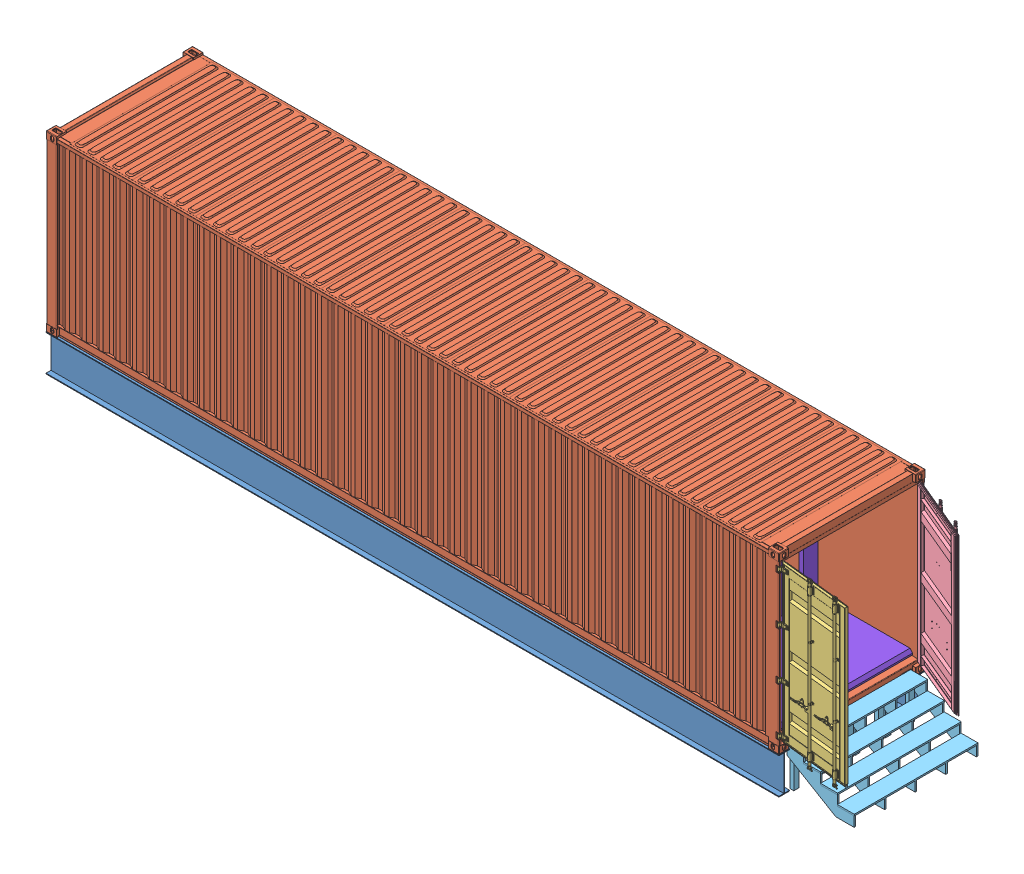
SolidWorks assembly Container - Top Level, configuration Default. Lengths in mm.
Overall size (13393.3 3505.2 2569.41).
30 component instances, 8 part files, 25 mates.
Components (placement in the parent):
- I-Beam-1: I-Beam [Default] at (-6096 -1759.7306 1147.032) x (0 0 1) z (-1 0 0) size (177.8 609.6 12192)
- I-Beam-2: I-Beam [Default] at (-6096 -1759.7306 -1113.1616) x (0 0 1) z (-1 0 0) size (177.8 609.6 12192)
- 40 ft. intermodal ISO Shipping container - BODY-1: 40 ft. intermodal ISO Shipping container - BODY [Default] at (-12190.6157 -1361.9436 1177.3313) size (12192 2895.6 2437.99)
- 40 ft. intermodal ISO Shipping container - LEFT DOOR-1: 40 ft. intermodal ISO Shipping container - LEFT DOOR [Default] at (-5430.0282 -1361.7966 -4818.236) x (-0.10789 0 0.994163) z (-0.994163 0 -0.10789) size (106.69 2751.15 1242.38)
- 40 ft. intermodal ISO Shipping container - RIGHT DOOR-1: 40 ft. intermodal ISO Shipping container - RIGHT DOOR [Default] at (-6294.5006 -1361.8704 5331.1159) x (0.387178 0.0003 -0.922005) z (0.922005 0.000375 0.387178) size (106.69 2751.11 1242.38)
- Stairs-1: Stairs [Default] at (-5035.4102 -2064.5306 -1011.7648) x (0 0 1) z (-1 0 0) size (2057.4 685.8 1120.77)
- MCM 64935T45 - PLANK GRATING-1: MCM 64935T45 - PLANK GRATING [18" Grate] at (-8486.1033 -1177.2343 -1113.3648) size (457.2 50.8 2260.6)
- MCM 64935T45 - PLANK GRATING-21: MCM 64935T45 - PLANK GRATING [12" Grate] at (-17687.2533 -1177.2343 -1113.3648) size (304.8 50.8 2260.6)
- MCM 64935T45 - PLANK GRATING-22: MCM 64935T45 - PLANK GRATING [12" Grate] at (-8092.4033 -1177.2343 -1113.3648) size (304.8 50.8 2260.6)
- MCM 64935T45 - PLANK GRATING-2: MCM 64935T45 - PLANK GRATING [18" Grate] at (-8949.6533 -1177.2343 -1113.3648) size (457.2 50.8 2260.6)
- MCM 64935T45 - PLANK GRATING-3: MCM 64935T45 - PLANK GRATING [18" Grate] at (-9413.2033 -1177.2343 -1113.3648) size (457.2 50.8 2260.6)
- MCM 64935T45 - PLANK GRATING-4: MCM 64935T45 - PLANK GRATING [18" Grate] at (-9876.7533 -1177.2343 -1113.3648) size (457.2 50.8 2260.6)
- MCM 64935T45 - PLANK GRATING-5: MCM 64935T45 - PLANK GRATING [18" Grate] at (-10340.3033 -1177.2343 -1113.3648) size (457.2 50.8 2260.6)
- MCM 64935T45 - PLANK GRATING-6: MCM 64935T45 - PLANK GRATING [18" Grate] at (-10803.8533 -1177.2343 -1113.3648) size (457.2 50.8 2260.6)
- MCM 64935T45 - PLANK GRATING-7: MCM 64935T45 - PLANK GRATING [18" Grate] at (-11267.4033 -1177.2343 -1113.3648) size (457.2 50.8 2260.6)
- MCM 64935T45 - PLANK GRATING-8: MCM 64935T45 - PLANK GRATING [18" Grate] at (-11730.9533 -1177.2343 -1113.3648) size (457.2 50.8 2260.6)
- MCM 64935T45 - PLANK GRATING-9: MCM 64935T45 - PLANK GRATING [18" Grate] at (-12194.5033 -1177.2343 -1113.3648) size (457.2 50.8 2260.6)
- MCM 64935T45 - PLANK GRATING-10: MCM 64935T45 - PLANK GRATING [18" Grate] at (-12658.0533 -1177.2343 -1113.3648) size (457.2 50.8 2260.6)
- MCM 64935T45 - PLANK GRATING-11: MCM 64935T45 - PLANK GRATING [18" Grate] at (-13121.6033 -1177.2343 -1113.3648) size (457.2 50.8 2260.6)
- MCM 64935T45 - PLANK GRATING-12: MCM 64935T45 - PLANK GRATING [18" Grate] at (-13585.1533 -1177.2343 -1113.3648) size (457.2 50.8 2260.6)
- MCM 64935T45 - PLANK GRATING-13: MCM 64935T45 - PLANK GRATING [18" Grate] at (-14048.7033 -1177.2343 -1113.3648) size (457.2 50.8 2260.6)
- MCM 64935T45 - PLANK GRATING-14: MCM 64935T45 - PLANK GRATING [18" Grate] at (-14512.2533 -1177.2343 -1113.3648) size (457.2 50.8 2260.6)
- MCM 64935T45 - PLANK GRATING-15: MCM 64935T45 - PLANK GRATING [18" Grate] at (-14975.8033 -1177.2343 -1113.3648) size (457.2 50.8 2260.6)
- MCM 64935T45 - PLANK GRATING-16: MCM 64935T45 - PLANK GRATING [18" Grate] at (-15439.3533 -1177.2343 -1113.3648) size (457.2 50.8 2260.6)
- MCM 64935T45 - PLANK GRATING-17: MCM 64935T45 - PLANK GRATING [18" Grate] at (-15902.9033 -1177.2343 -1113.3648) size (457.2 50.8 2260.6)
- MCM 64935T45 - PLANK GRATING-18: MCM 64935T45 - PLANK GRATING [18" Grate] at (-16366.4533 -1177.2343 -1113.3648) size (457.2 50.8 2260.6)
- MCM 64935T45 - PLANK GRATING-19: MCM 64935T45 - PLANK GRATING [18" Grate] at (-16830.0033 -1177.2343 -1113.3648) size (457.2 50.8 2260.6)
- MCM 64935T45 - PLANK GRATING-20: MCM 64935T45 - PLANK GRATING [18" Grate] at (-17293.5533 -1177.2343 -1113.3648) size (457.2 50.8 2260.6)
- Single Door Commercial Internal Left-1: Single Door Commercial Internal Left [Default] at (-7861.3 -1126.4343 477.3428) x (0 0 -1) z (1 0 0) size (1047.76 2203.46 229.66)
- Door Frame-1: Door Frame [Default] at (-7899.4 -34.2343 16.9678) x (0 0 -1) z (1 0 0) size (2311.4 2514.6 1651)
Mates (geometry in assembly coordinates):
- Lock1: lock: unknown of 40 ft. intermodal ISO Shipping container - LEFT DOOR-1; unknown of 40 ft. intermodal ISO Shipping container - BODY-1
- Lock2: lock: unknown of 40 ft. intermodal ISO Shipping container - BODY-1; unknown of ?
- Tangent2: tangent: face of 40 ft. intermodal ISO Shipping container - BODY-1; plane of I-Beam-1 through (-6096 -1759.7306 1147.032) normal (1 0 0)
- Tangent3: tangent: face of 40 ft. intermodal ISO Shipping container - BODY-1; plane of I-Beam-1 through (-18288 -1454.9306 1058.132) normal (0 1 0)
- Tangent4: tangent: face of 40 ft. intermodal ISO Shipping container - BODY-1; plane of I-Beam-1 through (-18288 -1454.9306 1235.932) normal (0 0 1)
- Coincident1: coincident: plane of I-Beam-1 through (-18288 -2064.5306 1235.932) normal (0 -1 0); plane of I-Beam-2 through (-18288 -2064.5306 -1024.2616) normal (0 -1 0)
- Tangent5: tangent: face of 40 ft. intermodal ISO Shipping container - BODY-1; plane of I-Beam-2 through (-18288 -1467.6306 -1202.0616) normal (0 0 -1)
- Coincident2: coincident: plane of I-Beam-1 through (-6096 -1759.7306 1147.032) normal (1 0 0); plane of I-Beam-2 through (-6096 -1759.7306 -1113.1616) normal (1 0 0)
- Tangent6: tangent: face of 40 ft. intermodal ISO Shipping container - BODY-1; plane of Stairs-1 through (-6153.0102 -1404.1306 -986.3648) normal (-1 0 0)
- Coincident3: coincident: plane of I-Beam-1 through (-18288 -2064.5306 1235.932) normal (0 -1 0); plane of Stairs-1 through (-5340.2102 -2064.5306 -986.3648) normal (0 -1 0)
- Width1: width: plane of Stairs-1 through (-5035.4102 -2064.5306 1045.6352) normal (0 0 1); plane of Stairs-1 through (-5035.4102 -2064.5306 -1011.7648) normal (0 0 -1); plane of I-Beam-1 through (-18288 -1467.6306 1140.682) normal (0 0 -1); plane of I-Beam-2 through (-18288 -1467.6306 -1106.8116) normal (0 0 1)
- Width2: width: plane of MCM 64935T45 - PLANK GRATING-1 through (-8267.0283 -1193.1093 1147.2352) normal (0 0 1); plane of MCM 64935T45 - PLANK GRATING-1 through (-8267.0283 -1193.1093 -1113.3648) normal (0 0 -1); plane of I-Beam-2 through (-18288 -1467.6306 -1119.5116) normal (0 0 -1); plane of I-Beam-1 through (-18288 -1467.6306 1153.382) normal (0 0 1)
- Distance1: distance = 2387.6 mm: plane of MCM 64935T45 - PLANK GRATING-1 through (-8705.1783 -1151.8343 1147.2352) normal (0 1 0); plane of 40 ft. intermodal ISO Shipping container - BODY-1 through (-6161.0102 1235.7657 1172.6678) normal (0 -1 0)
- Coincident4: coincident: plane of 40 ft. intermodal ISO Shipping container - BODY-1 through (-6161.0102 1235.7657 1172.6678) normal (0 -1 0); plane of Door Frame-1 through (-7823.2 1235.7657 1172.6678) normal (0 1 0)
- Width6: width: plane of Door Frame-1 through (-7823.2 1235.7657 -1138.7322) normal (0 0 -1); plane of Door Frame-1 through (-7823.2 1235.7657 1172.6678) normal (0 0 1); plane of 40 ft. intermodal ISO Shipping container - BODY-1 through (-6161.0102 1235.7657 -1138.7322) normal (0 0 1); plane of 40 ft. intermodal ISO Shipping container - BODY-1 through (-6161.0102 1235.7657 1172.6678) normal (0 0 -1)
- Coincident5: coincident: plane of Single Door Commercial Internal Left-1 through (-7823.2 -1126.4343 531.3178) normal (-1 0 0); plane of Door Frame-1 through (-7823.2 -34.2343 16.9678) normal (1 0 0)
- Coincident6: coincident: plane of Single Door Commercial Internal Left-1 through (-7861.3 1057.9657 1604.8702) normal (0 1 0); plane of Door Frame-1 through (-7823.2 1057.9657 524.9678) normal (0 -1 0)
- Coincident7: coincident: plane of Single Door Commercial Internal Left-1 through (-7861.3 -1126.4343 524.9678) normal (0 0 1); plane of Door Frame-1 through (-7823.2 1057.9657 524.9678) normal (0 0 -1)
- Distance2: distance = 1727.2 mm: plane of Door Frame-1 through (-7823.2 -34.2343 16.9678) normal (1 0 0); plane of I-Beam-1 through (-6096 -1759.7306 1147.032) normal (1 0 0)
- Coincident8: coincident: plane of MCM 64935T45 - PLANK GRATING-21 through (-17830.1283 -1151.8343 1147.2352) normal (0 1 0); plane of MCM 64935T45 - PLANK GRATING-22 through (-8235.2783 -1151.8343 1147.2352) normal (0 1 0)
- Coincident9: coincident: plane of MCM 64935T45 - PLANK GRATING-21 through (-17544.3783 -1193.1093 -1113.3648) normal (0 0 -1); plane of MCM 64935T45 - PLANK GRATING-22 through (-7949.5283 -1193.1093 -1113.3648) normal (0 0 -1)
- Coincident10: coincident: plane of MCM 64935T45 - PLANK GRATING-1 through (-8267.0283 -1193.1093 -1113.3648) normal (0 0 -1); plane of MCM 64935T45 - PLANK GRATING-21 through (-17544.3783 -1193.1093 -1113.3648) normal (0 0 -1)
- Coincident11: coincident: plane of MCM 64935T45 - PLANK GRATING-1 through (-8705.1783 -1151.8343 1147.2352) normal (0 1 0); plane of MCM 64935T45 - PLANK GRATING-21 through (-17830.1283 -1151.8343 1147.2352) normal (0 1 0)
- Distance3: distance = 12.7 mm: plane of MCM 64935T45 - PLANK GRATING-1 through (-8257.5033 -1161.3593 1147.2352) normal (1 0 0); plane of MCM 64935T45 - PLANK GRATING-22 through (-8244.8033 -1161.3593 1147.2352) normal (-1 0 0)
- Distance4: distance = 12.7 mm: plane of MCM 64935T45 - PLANK GRATING-21 through (-17534.8533 -1161.3593 1147.2352) normal (1 0 0); plane of MCM 64935T45 - PLANK GRATING-20 through (-17522.1533 -1161.3593 1147.2352) normal (-1 0 0)
